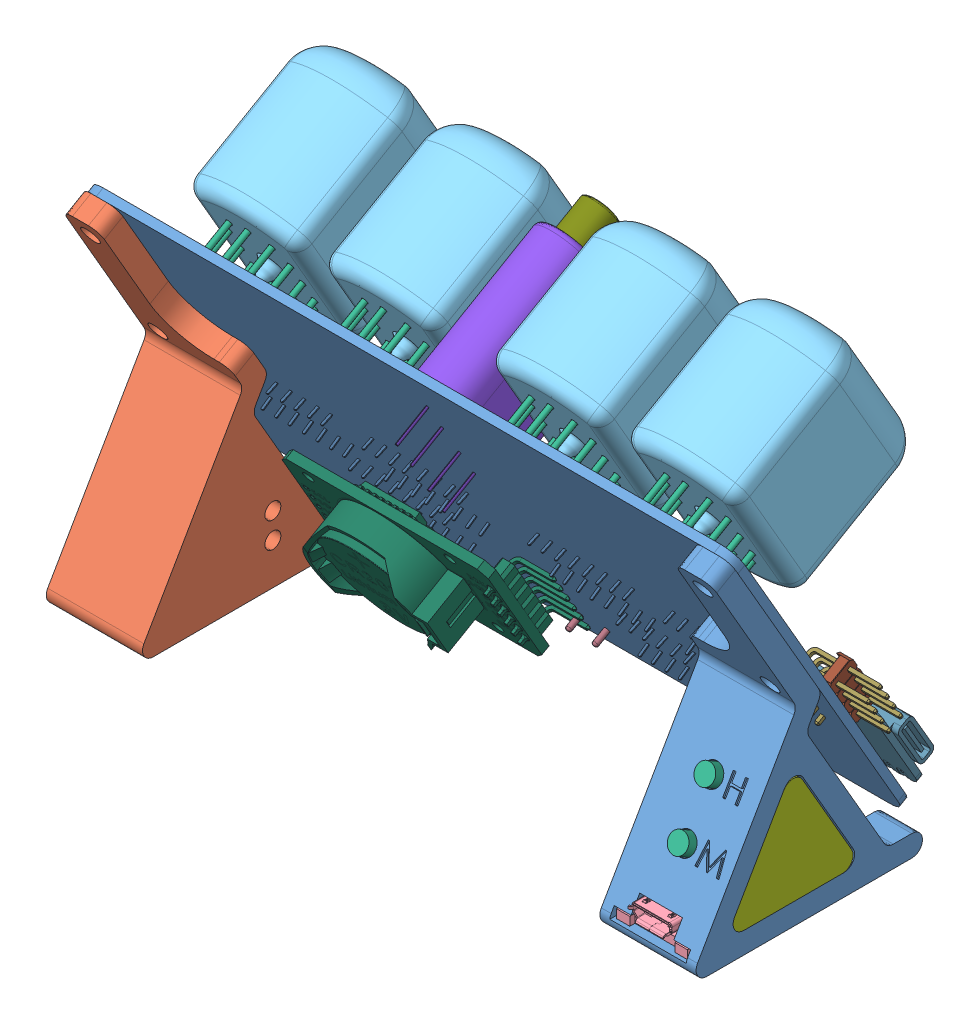
SolidWorks assembly assembly, configuration Défaut. Lengths in mm.
Overall size (130.66 87.93 77.4).
301 component instances, 62 part files, 34 mates.
Components (placement in the parent):
- board-1: board [Défaut] at (0 36.4164 17.774) x (-1 0 0) z (0 -0.866025 -0.5) size (127.16 50.53 67.27)
  - pcb-1: pcb [Défaut] at origin size (121.6 1.5 65.9)
  - IN-12A.stp-1: IN-12A.stp [Défaut] at (-40.9487 32.5 -15.5981) x (0 1 0) z (1 0 0) size (35 31 21)
    - 2.stp-1: 2.stp [Défaut] at origin size (2.7 24.17 15.83)
    - 3.stp-1: 3.stp [Défaut] at (-12.2 0 0) x (0 0 -1) z (-1 0 0) size (2 1.5 18.5)
    - 4.stp-1: 4.stp [Défaut] at (-12.2 0 0) x (0 0 1) z (-1 0 0) size (2 1.5 18.5)
    - 5.stp-1: 5.stp [Défaut] at (-12 0 0) x (0 0 -1) z (1 0 0) size (2.1 2.1 1)
    - 5.stp-2: 5.stp [Défaut] at (-10.8 0 0) x (0 0 -1) z (1 0 0) size (2.1 2.1 1)
    - 5.stp-3: 5.stp [Défaut] at (-9.6 0 0) x (0 0 -1) z (1 0 0) size (2.1 2.1 1)
    - 5.stp-4: 5.stp [Défaut] at (-8.4 0 0) x (0 0 -1) z (1 0 0) size (2.1 2.1 1)
    - 5.stp-5: 5.stp [Défaut] at (-7.2 0 0) x (0 0 -1) z (1 0 0) size (2.1 2.1 1)
    - 5.stp-6: 5.stp [Défaut] at (-6 0 0) x (0 0 -1) z (1 0 0) size (2.1 2.1 1)
    - 5.stp-7: 5.stp [Défaut] at (-4.8 0 0) x (0 0 -1) z (1 0 0) size (2.1 2.1 1)
    - 5.stp-8: 5.stp [Défaut] at (-3.6 0 0) x (0 0 -1) z (1 0 0) size (2.1 2.1 1)
    - 5.stp-9: 5.stp [Défaut] at (-2.4 0 0) x (0 0 -1) z (1 0 0) size (2.1 2.1 1)
    - 5.stp-10: 5.stp [Défaut] at (-1.2 0 0) x (0 0 -1) z (1 0 0) size (2.1 2.1 1)
    - 6.stp-1: 6.stp [Défaut] at (-11 16.1596 7.8778) x (0 -0.787778 0.61596) z (-1 0 0) size (2.1 2.1 1)
    - 7.stp-1: 7.stp [Défaut] at (-9.8 16.1596 7.8778) x (0 -0.787778 0.61596) z (-1 0 0) size (2.1 2.1 1)
    - 8.stp-1: 8.stp [Défaut] at (-8.6 16.1596 7.8778) x (0 -0.787778 0.61596) z (-1 0 0) size (2.1 2.1 1)
    - 9.stp-1: 9.stp [Défaut] at (-7.4 16.1596 7.8778) x (0 -0.787778 0.61596) z (-1 0 0) size (2.1 2.1 1)
    - 10.stp-1: 10.stp [Défaut] at (-6.2 16.1596 7.8778) x (0 -0.787778 0.61596) z (-1 0 0) size (2.1 2.1 1)
    - 11.stp-1: 11.stp [Défaut] at (-5 16.1596 7.8778) x (0 -0.787778 0.61596) z (-1 0 0) size (2.1 2.1 1)
    - 12.stp-1: 12.stp [Défaut] at (-3.8 16.1596 7.8778) x (0 -0.787778 0.61596) z (-1 0 0) size (2.1 2.1 1)
    - 13.stp-1: 13.stp [Défaut] at (-2.6 16.1596 7.8778) x (0 -0.787778 0.61596) z (-1 0 0) size (2.1 2.1 1)
    - 14.stp-1: 14.stp [Défaut] at (-1.4 16.1596 7.8778) x (0 -0.787778 0.61596) z (-1 0 0) size (2.1 2.1 1)
    - 15.stp-1: 15.stp [Défaut] at (-0.2 16.1596 7.8778) x (0 -0.787778 0.61596) z (-1 0 0) size (2.1 2.1 1)
    - 5.stp-11: 5.stp [Défaut] x (0 0 -1) z (1 0 0) size (2.1 2.1 1)
    - 5.stp-12: 5.stp [Défaut] at (-13.2 0 0) x (0 0 -1) z (1 0 0) size (2.1 2.1 1)
    - 16.stp-1: 16.stp [Défaut] at (1 16.1596 7.8778) x (0 -0.787778 0.61596) z (-1 0 0) size (2.1 2.1 1)
    - 17.stp-1: 17.stp [Défaut] at (-12.2 16.1596 7.8778) x (0 -0.787778 0.61596) z (-1 0 0) size (2.1 2.1 1)
    - 18.stp-1: 18.stp [Défaut] at (-13.2 0 0) x (0 0 -1) z (-1 0 0) size (15.83 24.17 12.28)
    - 19.stp-1: 19.stp [Défaut] x (1 0 0) z (0 1 0) size (1.51 1.46 20.68)
    - 20.stp-1: 20.stp [Défaut] at (1 0 0) size (4 22.27 2.42)
    - 21.stp-1: 21.stp [Défaut] at (-13.4 0 0) x (0 0 -1) z (-1 0 0) size (15.83 24.17 1)
    - 22.stp-1: 22.stp [Défaut] at (-14.4 0 0) x (0 0 -1) z (-1 0 0) size (15.83 27.29 2)
    - 23.stp-1: 23.stp [Défaut] x (0 0 -1) z (-1 0 0) size (21 31 33)
    - 24.stp-1: 24.stp [Défaut] x (0 0 -1) z (-1 0 0) size (1 1 15.5)
    - 24.stp-2: 24.stp [Défaut] at (0 -4.5 0) x (0 0 -1) z (-1 0 0) size (1 1 15.5)
    - 24.stp-3: 24.stp [Défaut] at (0 -8 -1.75) x (0 0 -1) z (-1 0 0) size (1 1 15.5)
    - 24.stp-4: 24.stp [Défaut] at (0 -9 -5.75) x (0 0 -1) z (-1 0 0) size (1 1 15.5)
    - 24.stp-5: 24.stp [Défaut] at (0 -8 -9.75) x (0 0 -1) z (-1 0 0) size (1 1 15.5)
    - 24.stp-6: 24.stp [Défaut] at (0 -4.5 -11.5) x (0 0 -1) z (-1 0 0) size (1 1 15.5)
    - 24.stp-7: 24.stp [Défaut] at (0 0 -11.5) x (0 0 -1) z (-1 0 0) size (1 1 15.5)
    - 24.stp-8: 24.stp [Défaut] at (0 4.5 -11.5) x (0 0 -1) z (-1 0 0) size (1 1 15.5)
    - 24.stp-9: 24.stp [Défaut] at (0 8 -9.75) x (0 0 -1) z (-1 0 0) size (1 1 15.5)
    - 24.stp-10: 24.stp [Défaut] at (0 9 -5.75) x (0 0 -1) z (-1 0 0) size (1 1 15.5)
    - 24.stp-11: 24.stp [Défaut] at (0 8 -1.75) x (0 0 -1) z (-1 0 0) size (1 1 15.5)
    - 24.stp-12: 24.stp [Défaut] at (0 4.5 0) x (0 0 -1) z (-1 0 0) size (1 1 15.5)
    - 25.stp-1: 25.stp [Défaut] at (-1.4 0 0) x (0 0 1) z (1 0 0) size (10.55 22 0.2)
    - 26.stp-1: 26.stp [Défaut] at (-2.6 0 0) x (0 0 1) z (1 0 0) size (11 22 0.2)
    - 27.stp-1: 27.stp [Défaut] at (-3.8 0 0) x (0 0 1) z (1 0 0) size (11 22 0.2)
    - 28.stp-1: 28.stp [Défaut] at (-5 0 0) x (0 0 1) z (1 0 0) size (10 22 0.2)
    - 29.stp-1: 29.stp [Défaut] at (-7.4 0 0) x (0 0 1) z (1 0 0) size (10 22 0.2)
    - 30.stp-1: 30.stp [Défaut] at (-9.6 0 0) x (0 0 -1) z (-1 0 0) size (10 22 0.2)
    - 31.stp-1: 31.stp [Défaut] at (-11 0 0) x (0 0 1) z (1 0 0) size (11 22 0.2)
    - 32.stp-1: 32.stp [Défaut] at (-12.2 0 0) x (0 0 1) z (1 0 0) size (2 22 0.2)
    - 33.stp-1: 33.stp [Défaut] at (-6 0 0) x (0 0 -1) z (-1 0 0) size (11 22 0.2)
    - 34.stp-1: 34.stp [Défaut] at (-8.6 0 0) x (0 0 1) z (1 0 0) size (10 22 0.2)
    - 1.stp-1: 1.stp [Défaut] at origin size (7.54 3.19 3.19)
    - 1-0.stp-1: 1-0.stp [Défaut] at origin size (11.99 9.11 6.32)
    - 1-1.stp-1: 1-1.stp [Défaut] at origin size (5.03 4.26 4.61)
    - 1-2.stp-1: 1-2.stp [Défaut] at origin size (8.17 8.42 6.65)
    - 1-3.stp-1: 1-3.stp [Défaut] at origin size (17.22 12.89 7.69)
    - 1-4.stp-1: 1-4.stp [Défaut] at origin size (13.11 12.81 7.39)
    - 1-5.stp-1: 1-5.stp [Défaut] at origin size (15.91 7.54 6.9)
    - 1-6.stp-1: 1-6.stp [Défaut] at origin size (10.39 4.47 4.23)
    - 1-7.stp-1: 1-7.stp [Défaut] at origin size (7.32 4.98 2.44)
    - 1-8.stp-1: 1-8.stp [Défaut] at origin size (10.29 4.36 5.63)
    - 1-9.stp-1: 1-9.stp [Défaut] at origin size (12.89 8.1 7.83)
  - IN-12A.stp-2: IN-12A.stp [Défaut] at (15.5408 32.5 -15.6508) x (0 1 0) z (1 0 0) size (35 31 21)
    - 2.stp-1: 2.stp [Défaut] at origin size (2.7 24.17 15.83)
    - 3.stp-1: 3.stp [Défaut] at (-12.2 0 0) x (0 0 -1) z (-1 0 0) size (2 1.5 18.5)
    - 4.stp-1: 4.stp [Défaut] at (-12.2 0 0) x (0 0 1) z (-1 0 0) size (2 1.5 18.5)
    - 5.stp-1: 5.stp [Défaut] at (-12 0 0) x (0 0 -1) z (1 0 0) size (2.1 2.1 1)
    - 5.stp-2: 5.stp [Défaut] at (-10.8 0 0) x (0 0 -1) z (1 0 0) size (2.1 2.1 1)
    - 5.stp-3: 5.stp [Défaut] at (-9.6 0 0) x (0 0 -1) z (1 0 0) size (2.1 2.1 1)
    - 5.stp-4: 5.stp [Défaut] at (-8.4 0 0) x (0 0 -1) z (1 0 0) size (2.1 2.1 1)
    - 5.stp-5: 5.stp [Défaut] at (-7.2 0 0) x (0 0 -1) z (1 0 0) size (2.1 2.1 1)
    - 5.stp-6: 5.stp [Défaut] at (-6 0 0) x (0 0 -1) z (1 0 0) size (2.1 2.1 1)
    - 5.stp-7: 5.stp [Défaut] at (-4.8 0 0) x (0 0 -1) z (1 0 0) size (2.1 2.1 1)
    - 5.stp-8: 5.stp [Défaut] at (-3.6 0 0) x (0 0 -1) z (1 0 0) size (2.1 2.1 1)
    - 5.stp-9: 5.stp [Défaut] at (-2.4 0 0) x (0 0 -1) z (1 0 0) size (2.1 2.1 1)
    - 5.stp-10: 5.stp [Défaut] at (-1.2 0 0) x (0 0 -1) z (1 0 0) size (2.1 2.1 1)
    - 6.stp-1: 6.stp [Défaut] at (-11 16.1596 7.8778) x (0 -0.787778 0.61596) z (-1 0 0) size (2.1 2.1 1)
    - 7.stp-1: 7.stp [Défaut] at (-9.8 16.1596 7.8778) x (0 -0.787778 0.61596) z (-1 0 0) size (2.1 2.1 1)
    - 8.stp-1: 8.stp [Défaut] at (-8.6 16.1596 7.8778) x (0 -0.787778 0.61596) z (-1 0 0) size (2.1 2.1 1)
    - 9.stp-1: 9.stp [Défaut] at (-7.4 16.1596 7.8778) x (0 -0.787778 0.61596) z (-1 0 0) size (2.1 2.1 1)
    - 10.stp-1: 10.stp [Défaut] at (-6.2 16.1596 7.8778) x (0 -0.787778 0.61596) z (-1 0 0) size (2.1 2.1 1)
    - 11.stp-1: 11.stp [Défaut] at (-5 16.1596 7.8778) x (0 -0.787778 0.61596) z (-1 0 0) size (2.1 2.1 1)
    - 12.stp-1: 12.stp [Défaut] at (-3.8 16.1596 7.8778) x (0 -0.787778 0.61596) z (-1 0 0) size (2.1 2.1 1)
    - 13.stp-1: 13.stp [Défaut] at (-2.6 16.1596 7.8778) x (0 -0.787778 0.61596) z (-1 0 0) size (2.1 2.1 1)
    - 14.stp-1: 14.stp [Défaut] at (-1.4 16.1596 7.8778) x (0 -0.787778 0.61596) z (-1 0 0) size (2.1 2.1 1)
    - 15.stp-1: 15.stp [Défaut] at (-0.2 16.1596 7.8778) x (0 -0.787778 0.61596) z (-1 0 0) size (2.1 2.1 1)
    - 5.stp-11: 5.stp [Défaut] x (0 0 -1) z (1 0 0) size (2.1 2.1 1)
    - 5.stp-12: 5.stp [Défaut] at (-13.2 0 0) x (0 0 -1) z (1 0 0) size (2.1 2.1 1)
    - 16.stp-1: 16.stp [Défaut] at (1 16.1596 7.8778) x (0 -0.787778 0.61596) z (-1 0 0) size (2.1 2.1 1)
    - 17.stp-1: 17.stp [Défaut] at (-12.2 16.1596 7.8778) x (0 -0.787778 0.61596) z (-1 0 0) size (2.1 2.1 1)
    - 18.stp-1: 18.stp [Défaut] at (-13.2 0 0) x (0 0 -1) z (-1 0 0) size (15.83 24.17 12.28)
    - 19.stp-1: 19.stp [Défaut] x (1 0 0) z (0 1 0) size (1.51 1.46 20.68)
    - 20.stp-1: 20.stp [Défaut] at (1 0 0) size (4 22.27 2.42)
    - 21.stp-1: 21.stp [Défaut] at (-13.4 0 0) x (0 0 -1) z (-1 0 0) size (15.83 24.17 1)
    - 22.stp-1: 22.stp [Défaut] at (-14.4 0 0) x (0 0 -1) z (-1 0 0) size (15.83 27.29 2)
    - 23.stp-1: 23.stp [Défaut] x (0 0 -1) z (-1 0 0) size (21 31 33)
    - 24.stp-1: 24.stp [Défaut] x (0 0 -1) z (-1 0 0) size (1 1 15.5)
    - 24.stp-2: 24.stp [Défaut] at (0 -4.5 0) x (0 0 -1) z (-1 0 0) size (1 1 15.5)
    - 24.stp-3: 24.stp [Défaut] at (0 -8 -1.75) x (0 0 -1) z (-1 0 0) size (1 1 15.5)
    - 24.stp-4: 24.stp [Défaut] at (0 -9 -5.75) x (0 0 -1) z (-1 0 0) size (1 1 15.5)
    - 24.stp-5: 24.stp [Défaut] at (0 -8 -9.75) x (0 0 -1) z (-1 0 0) size (1 1 15.5)
    - 24.stp-6: 24.stp [Défaut] at (0 -4.5 -11.5) x (0 0 -1) z (-1 0 0) size (1 1 15.5)
    - 24.stp-7: 24.stp [Défaut] at (0 0 -11.5) x (0 0 -1) z (-1 0 0) size (1 1 15.5)
    - 24.stp-8: 24.stp [Défaut] at (0 4.5 -11.5) x (0 0 -1) z (-1 0 0) size (1 1 15.5)
    - 24.stp-9: 24.stp [Défaut] at (0 8 -9.75) x (0 0 -1) z (-1 0 0) size (1 1 15.5)
    - 24.stp-10: 24.stp [Défaut] at (0 9 -5.75) x (0 0 -1) z (-1 0 0) size (1 1 15.5)
    - 24.stp-11: 24.stp [Défaut] at (0 8 -1.75) x (0 0 -1) z (-1 0 0) size (1 1 15.5)
    - 24.stp-12: 24.stp [Défaut] at (0 4.5 0) x (0 0 -1) z (-1 0 0) size (1 1 15.5)
    - 25.stp-1: 25.stp [Défaut] at (-1.4 0 0) x (0 0 1) z (1 0 0) size (10.55 22 0.2)
    - 26.stp-1: 26.stp [Défaut] at (-2.6 0 0) x (0 0 1) z (1 0 0) size (11 22 0.2)
    - 27.stp-1: 27.stp [Défaut] at (-3.8 0 0) x (0 0 1) z (1 0 0) size (11 22 0.2)
    - 28.stp-1: 28.stp [Défaut] at (-5 0 0) x (0 0 1) z (1 0 0) size (10 22 0.2)
    - 29.stp-1: 29.stp [Défaut] at (-7.4 0 0) x (0 0 1) z (1 0 0) size (10 22 0.2)
    - 30.stp-1: 30.stp [Défaut] at (-9.6 0 0) x (0 0 -1) z (-1 0 0) size (10 22 0.2)
    - 31.stp-1: 31.stp [Défaut] at (-11 0 0) x (0 0 1) z (1 0 0) size (11 22 0.2)
    - 32.stp-1: 32.stp [Défaut] at (-12.2 0 0) x (0 0 1) z (1 0 0) size (2 22 0.2)
    - 33.stp-1: 33.stp [Défaut] at (-6 0 0) x (0 0 -1) z (-1 0 0) size (11 22 0.2)
    - 34.stp-1: 34.stp [Défaut] at (-8.6 0 0) x (0 0 1) z (1 0 0) size (10 22 0.2)
    - 1.stp-1: 1.stp [Défaut] at origin size (7.54 3.19 3.19)
    - 1-0.stp-1: 1-0.stp [Défaut] at origin size (11.99 9.11 6.32)
    - 1-1.stp-1: 1-1.stp [Défaut] at origin size (5.03 4.26 4.61)
    - 1-2.stp-1: 1-2.stp [Défaut] at origin size (8.17 8.42 6.65)
    - 1-3.stp-1: 1-3.stp [Défaut] at origin size (17.22 12.89 7.69)
    - 1-4.stp-1: 1-4.stp [Défaut] at origin size (13.11 12.81 7.39)
    - 1-5.stp-1: 1-5.stp [Défaut] at origin size (15.91 7.54 6.9)
    - 1-6.stp-1: 1-6.stp [Défaut] at origin size (10.39 4.47 4.23)
    - 1-7.stp-1: 1-7.stp [Défaut] at origin size (7.32 4.98 2.44)
    - 1-8.stp-1: 1-8.stp [Défaut] at origin size (10.29 4.36 5.63)
    - 1-9.stp-1: 1-9.stp [Défaut] at origin size (12.89 8.1 7.83)
  - IN-12A.stp-3: IN-12A.stp [Défaut] at (-15.577 32.5 -15.4564) x (0 1 0) z (1 0 0) size (35 31 21)
    - 2.stp-1: 2.stp [Défaut] at origin size (2.7 24.17 15.83)
    - 3.stp-1: 3.stp [Défaut] at (-12.2 0 0) x (0 0 -1) z (-1 0 0) size (2 1.5 18.5)
    - 4.stp-1: 4.stp [Défaut] at (-12.2 0 0) x (0 0 1) z (-1 0 0) size (2 1.5 18.5)
    - 5.stp-1: 5.stp [Défaut] at (-12 0 0) x (0 0 -1) z (1 0 0) size (2.1 2.1 1)
    - 5.stp-2: 5.stp [Défaut] at (-10.8 0 0) x (0 0 -1) z (1 0 0) size (2.1 2.1 1)
    - 5.stp-3: 5.stp [Défaut] at (-9.6 0 0) x (0 0 -1) z (1 0 0) size (2.1 2.1 1)
    - 5.stp-4: 5.stp [Défaut] at (-8.4 0 0) x (0 0 -1) z (1 0 0) size (2.1 2.1 1)
    - 5.stp-5: 5.stp [Défaut] at (-7.2 0 0) x (0 0 -1) z (1 0 0) size (2.1 2.1 1)
    - 5.stp-6: 5.stp [Défaut] at (-6 0 0) x (0 0 -1) z (1 0 0) size (2.1 2.1 1)
    - 5.stp-7: 5.stp [Défaut] at (-4.8 0 0) x (0 0 -1) z (1 0 0) size (2.1 2.1 1)
    - 5.stp-8: 5.stp [Défaut] at (-3.6 0 0) x (0 0 -1) z (1 0 0) size (2.1 2.1 1)
    - 5.stp-9: 5.stp [Défaut] at (-2.4 0 0) x (0 0 -1) z (1 0 0) size (2.1 2.1 1)
    - 5.stp-10: 5.stp [Défaut] at (-1.2 0 0) x (0 0 -1) z (1 0 0) size (2.1 2.1 1)
    - 6.stp-1: 6.stp [Défaut] at (-11 16.1596 7.8778) x (0 -0.787778 0.61596) z (-1 0 0) size (2.1 2.1 1)
    - 7.stp-1: 7.stp [Défaut] at (-9.8 16.1596 7.8778) x (0 -0.787778 0.61596) z (-1 0 0) size (2.1 2.1 1)
    - 8.stp-1: 8.stp [Défaut] at (-8.6 16.1596 7.8778) x (0 -0.787778 0.61596) z (-1 0 0) size (2.1 2.1 1)
    - 9.stp-1: 9.stp [Défaut] at (-7.4 16.1596 7.8778) x (0 -0.787778 0.61596) z (-1 0 0) size (2.1 2.1 1)
    - 10.stp-1: 10.stp [Défaut] at (-6.2 16.1596 7.8778) x (0 -0.787778 0.61596) z (-1 0 0) size (2.1 2.1 1)
    - 11.stp-1: 11.stp [Défaut] at (-5 16.1596 7.8778) x (0 -0.787778 0.61596) z (-1 0 0) size (2.1 2.1 1)
    - 12.stp-1: 12.stp [Défaut] at (-3.8 16.1596 7.8778) x (0 -0.787778 0.61596) z (-1 0 0) size (2.1 2.1 1)
    - 13.stp-1: 13.stp [Défaut] at (-2.6 16.1596 7.8778) x (0 -0.787778 0.61596) z (-1 0 0) size (2.1 2.1 1)
    - 14.stp-1: 14.stp [Défaut] at (-1.4 16.1596 7.8778) x (0 -0.787778 0.61596) z (-1 0 0) size (2.1 2.1 1)
    - 15.stp-1: 15.stp [Défaut] at (-0.2 16.1596 7.8778) x (0 -0.787778 0.61596) z (-1 0 0) size (2.1 2.1 1)
    - 5.stp-11: 5.stp [Défaut] x (0 0 -1) z (1 0 0) size (2.1 2.1 1)
    - 5.stp-12: 5.stp [Défaut] at (-13.2 0 0) x (0 0 -1) z (1 0 0) size (2.1 2.1 1)
    - 16.stp-1: 16.stp [Défaut] at (1 16.1596 7.8778) x (0 -0.787778 0.61596) z (-1 0 0) size (2.1 2.1 1)
    - 17.stp-1: 17.stp [Défaut] at (-12.2 16.1596 7.8778) x (0 -0.787778 0.61596) z (-1 0 0) size (2.1 2.1 1)
    - 18.stp-1: 18.stp [Défaut] at (-13.2 0 0) x (0 0 -1) z (-1 0 0) size (15.83 24.17 12.28)
    - 19.stp-1: 19.stp [Défaut] x (1 0 0) z (0 1 0) size (1.51 1.46 20.68)
    - 20.stp-1: 20.stp [Défaut] at (1 0 0) size (4 22.27 2.42)
    - 21.stp-1: 21.stp [Défaut] at (-13.4 0 0) x (0 0 -1) z (-1 0 0) size (15.83 24.17 1)
    - 22.stp-1: 22.stp [Défaut] at (-14.4 0 0) x (0 0 -1) z (-1 0 0) size (15.83 27.29 2)
    - 23.stp-1: 23.stp [Défaut] x (0 0 -1) z (-1 0 0) size (21 31 33)
    - 24.stp-1: 24.stp [Défaut] x (0 0 -1) z (-1 0 0) size (1 1 15.5)
    - 24.stp-2: 24.stp [Défaut] at (0 -4.5 0) x (0 0 -1) z (-1 0 0) size (1 1 15.5)
    - 24.stp-3: 24.stp [Défaut] at (0 -8 -1.75) x (0 0 -1) z (-1 0 0) size (1 1 15.5)
    - 24.stp-4: 24.stp [Défaut] at (0 -9 -5.75) x (0 0 -1) z (-1 0 0) size (1 1 15.5)
    - 24.stp-5: 24.stp [Défaut] at (0 -8 -9.75) x (0 0 -1) z (-1 0 0) size (1 1 15.5)
    - 24.stp-6: 24.stp [Défaut] at (0 -4.5 -11.5) x (0 0 -1) z (-1 0 0) size (1 1 15.5)
    - 24.stp-7: 24.stp [Défaut] at (0 0 -11.5) x (0 0 -1) z (-1 0 0) size (1 1 15.5)
    - 24.stp-8: 24.stp [Défaut] at (0 4.5 -11.5) x (0 0 -1) z (-1 0 0) size (1 1 15.5)
    - 24.stp-9: 24.stp [Défaut] at (0 8 -9.75) x (0 0 -1) z (-1 0 0) size (1 1 15.5)
    - 24.stp-10: 24.stp [Défaut] at (0 9 -5.75) x (0 0 -1) z (-1 0 0) size (1 1 15.5)
    - 24.stp-11: 24.stp [Défaut] at (0 8 -1.75) x (0 0 -1) z (-1 0 0) size (1 1 15.5)
    - 24.stp-12: 24.stp [Défaut] at (0 4.5 0) x (0 0 -1) z (-1 0 0) size (1 1 15.5)
    - 25.stp-1: 25.stp [Défaut] at (-1.4 0 0) x (0 0 1) z (1 0 0) size (10.55 22 0.2)
    - 26.stp-1: 26.stp [Défaut] at (-2.6 0 0) x (0 0 1) z (1 0 0) size (11 22 0.2)
    - 27.stp-1: 27.stp [Défaut] at (-3.8 0 0) x (0 0 1) z (1 0 0) size (11 22 0.2)
    - 28.stp-1: 28.stp [Défaut] at (-5 0 0) x (0 0 1) z (1 0 0) size (10 22 0.2)
    - 29.stp-1: 29.stp [Défaut] at (-7.4 0 0) x (0 0 1) z (1 0 0) size (10 22 0.2)
    - 30.stp-1: 30.stp [Défaut] at (-9.6 0 0) x (0 0 -1) z (-1 0 0) size (10 22 0.2)
    - 31.stp-1: 31.stp [Défaut] at (-11 0 0) x (0 0 1) z (1 0 0) size (11 22 0.2)
    - 32.stp-1: 32.stp [Défaut] at (-12.2 0 0) x (0 0 1) z (1 0 0) size (2 22 0.2)
    - 33.stp-1: 33.stp [Défaut] at (-6 0 0) x (0 0 -1) z (-1 0 0) size (11 22 0.2)
    - 34.stp-1: 34.stp [Défaut] at (-8.6 0 0) x (0 0 1) z (1 0 0) size (10 22 0.2)
    - 1.stp-1: 1.stp [Défaut] at origin size (7.54 3.19 3.19)
    - 1-0.stp-1: 1-0.stp [Défaut] at origin size (11.99 9.11 6.32)
    - 1-1.stp-1: 1-1.stp [Défaut] at origin size (5.03 4.26 4.61)
    - 1-2.stp-1: 1-2.stp [Défaut] at origin size (8.17 8.42 6.65)
    - 1-3.stp-1: 1-3.stp [Défaut] at origin size (17.22 12.89 7.69)
    - 1-4.stp-1: 1-4.stp [Défaut] at origin size (13.11 12.81 7.39)
    - 1-5.stp-1: 1-5.stp [Défaut] at origin size (15.91 7.54 6.9)
    - 1-6.stp-1: 1-6.stp [Défaut] at origin size (10.39 4.47 4.23)
    - 1-7.stp-1: 1-7.stp [Défaut] at origin size (7.32 4.98 2.44)
    - 1-8.stp-1: 1-8.stp [Défaut] at origin size (10.29 4.36 5.63)
    - 1-9.stp-1: 1-9.stp [Défaut] at origin size (12.89 8.1 7.83)
  - IN-12A.stp-4: IN-12A.stp [Défaut] at (40.934 32.5 -15.666) x (0 1 0) z (1 0 0) size (35 31 21)
    - 2.stp-1: 2.stp [Défaut] at origin size (2.7 24.17 15.83)
    - 3.stp-1: 3.stp [Défaut] at (-12.2 0 0) x (0 0 -1) z (-1 0 0) size (2 1.5 18.5)
    - 4.stp-1: 4.stp [Défaut] at (-12.2 0 0) x (0 0 1) z (-1 0 0) size (2 1.5 18.5)
    - 5.stp-1: 5.stp [Défaut] at (-12 0 0) x (0 0 -1) z (1 0 0) size (2.1 2.1 1)
    - 5.stp-2: 5.stp [Défaut] at (-10.8 0 0) x (0 0 -1) z (1 0 0) size (2.1 2.1 1)
    - 5.stp-3: 5.stp [Défaut] at (-9.6 0 0) x (0 0 -1) z (1 0 0) size (2.1 2.1 1)
    - 5.stp-4: 5.stp [Défaut] at (-8.4 0 0) x (0 0 -1) z (1 0 0) size (2.1 2.1 1)
    - 5.stp-5: 5.stp [Défaut] at (-7.2 0 0) x (0 0 -1) z (1 0 0) size (2.1 2.1 1)
    - 5.stp-6: 5.stp [Défaut] at (-6 0 0) x (0 0 -1) z (1 0 0) size (2.1 2.1 1)
    - 5.stp-7: 5.stp [Défaut] at (-4.8 0 0) x (0 0 -1) z (1 0 0) size (2.1 2.1 1)
    - 5.stp-8: 5.stp [Défaut] at (-3.6 0 0) x (0 0 -1) z (1 0 0) size (2.1 2.1 1)
    - 5.stp-9: 5.stp [Défaut] at (-2.4 0 0) x (0 0 -1) z (1 0 0) size (2.1 2.1 1)
    - 5.stp-10: 5.stp [Défaut] at (-1.2 0 0) x (0 0 -1) z (1 0 0) size (2.1 2.1 1)
    - 6.stp-1: 6.stp [Défaut] at (-11 16.1596 7.8778) x (0 -0.787778 0.61596) z (-1 0 0) size (2.1 2.1 1)
    - 7.stp-1: 7.stp [Défaut] at (-9.8 16.1596 7.8778) x (0 -0.787778 0.61596) z (-1 0 0) size (2.1 2.1 1)
    - 8.stp-1: 8.stp [Défaut] at (-8.6 16.1596 7.8778) x (0 -0.787778 0.61596) z (-1 0 0) size (2.1 2.1 1)
    - 9.stp-1: 9.stp [Défaut] at (-7.4 16.1596 7.8778) x (0 -0.787778 0.61596) z (-1 0 0) size (2.1 2.1 1)
    - 10.stp-1: 10.stp [Défaut] at (-6.2 16.1596 7.8778) x (0 -0.787778 0.61596) z (-1 0 0) size (2.1 2.1 1)
    - 11.stp-1: 11.stp [Défaut] at (-5 16.1596 7.8778) x (0 -0.787778 0.61596) z (-1 0 0) size (2.1 2.1 1)
    - 12.stp-1: 12.stp [Défaut] at (-3.8 16.1596 7.8778) x (0 -0.787778 0.61596) z (-1 0 0) size (2.1 2.1 1)
    - 13.stp-1: 13.stp [Défaut] at (-2.6 16.1596 7.8778) x (0 -0.787778 0.61596) z (-1 0 0) size (2.1 2.1 1)
    - 14.stp-1: 14.stp [Défaut] at (-1.4 16.1596 7.8778) x (0 -0.787778 0.61596) z (-1 0 0) size (2.1 2.1 1)
    - 15.stp-1: 15.stp [Défaut] at (-0.2 16.1596 7.8778) x (0 -0.787778 0.61596) z (-1 0 0) size (2.1 2.1 1)
    - 5.stp-11: 5.stp [Défaut] x (0 0 -1) z (1 0 0) size (2.1 2.1 1)
    - 5.stp-12: 5.stp [Défaut] at (-13.2 0 0) x (0 0 -1) z (1 0 0) size (2.1 2.1 1)
    - 16.stp-1: 16.stp [Défaut] at (1 16.1596 7.8778) x (0 -0.787778 0.61596) z (-1 0 0) size (2.1 2.1 1)
    - 17.stp-1: 17.stp [Défaut] at (-12.2 16.1596 7.8778) x (0 -0.787778 0.61596) z (-1 0 0) size (2.1 2.1 1)
    - 18.stp-1: 18.stp [Défaut] at (-13.2 0 0) x (0 0 -1) z (-1 0 0) size (15.83 24.17 12.28)
    - 19.stp-1: 19.stp [Défaut] x (1 0 0) z (0 1 0) size (1.51 1.46 20.68)
    - 20.stp-1: 20.stp [Défaut] at (1 0 0) size (4 22.27 2.42)
    - 21.stp-1: 21.stp [Défaut] at (-13.4 0 0) x (0 0 -1) z (-1 0 0) size (15.83 24.17 1)
    - 22.stp-1: 22.stp [Défaut] at (-14.4 0 0) x (0 0 -1) z (-1 0 0) size (15.83 27.29 2)
    - 23.stp-1: 23.stp [Défaut] x (0 0 -1) z (-1 0 0) size (21 31 33)
    - 24.stp-1: 24.stp [Défaut] x (0 0 -1) z (-1 0 0) size (1 1 15.5)
    - 24.stp-2: 24.stp [Défaut] at (0 -4.5 0) x (0 0 -1) z (-1 0 0) size (1 1 15.5)
    - 24.stp-3: 24.stp [Défaut] at (0 -8 -1.75) x (0 0 -1) z (-1 0 0) size (1 1 15.5)
    - 24.stp-4: 24.stp [Défaut] at (0 -9 -5.75) x (0 0 -1) z (-1 0 0) size (1 1 15.5)
    - 24.stp-5: 24.stp [Défaut] at (0 -8 -9.75) x (0 0 -1) z (-1 0 0) size (1 1 15.5)
    - 24.stp-6: 24.stp [Défaut] at (0 -4.5 -11.5) x (0 0 -1) z (-1 0 0) size (1 1 15.5)
    - 24.stp-7: 24.stp [Défaut] at (0 0 -11.5) x (0 0 -1) z (-1 0 0) size (1 1 15.5)
    - 24.stp-8: 24.stp [Défaut] at (0 4.5 -11.5) x (0 0 -1) z (-1 0 0) size (1 1 15.5)
    - 24.stp-9: 24.stp [Défaut] at (0 8 -9.75) x (0 0 -1) z (-1 0 0) size (1 1 15.5)
    - 24.stp-10: 24.stp [Défaut] at (0 9 -5.75) x (0 0 -1) z (-1 0 0) size (1 1 15.5)
    - 24.stp-11: 24.stp [Défaut] at (0 8 -1.75) x (0 0 -1) z (-1 0 0) size (1 1 15.5)
    - 24.stp-12: 24.stp [Défaut] at (0 4.5 0) x (0 0 -1) z (-1 0 0) size (1 1 15.5)
    - 25.stp-1: 25.stp [Défaut] at (-1.4 0 0) x (0 0 1) z (1 0 0) size (10.55 22 0.2)
    - 26.stp-1: 26.stp [Défaut] at (-2.6 0 0) x (0 0 1) z (1 0 0) size (11 22 0.2)
    - 27.stp-1: 27.stp [Défaut] at (-3.8 0 0) x (0 0 1) z (1 0 0) size (11 22 0.2)
    - 28.stp-1: 28.stp [Défaut] at (-5 0 0) x (0 0 1) z (1 0 0) size (10 22 0.2)
    - 29.stp-1: 29.stp [Défaut] at (-7.4 0 0) x (0 0 1) z (1 0 0) size (10 22 0.2)
    - 30.stp-1: 30.stp [Défaut] at (-9.6 0 0) x (0 0 -1) z (-1 0 0) size (10 22 0.2)
    - 31.stp-1: 31.stp [Défaut] at (-11 0 0) x (0 0 1) z (1 0 0) size (11 22 0.2)
    - 32.stp-1: 32.stp [Défaut] at (-12.2 0 0) x (0 0 1) z (1 0 0) size (2 22 0.2)
    - 33.stp-1: 33.stp [Défaut] at (-6 0 0) x (0 0 -1) z (-1 0 0) size (11 22 0.2)
    - 34.stp-1: 34.stp [Défaut] at (-8.6 0 0) x (0 0 1) z (1 0 0) size (10 22 0.2)
    - 1.stp-1: 1.stp [Défaut] at origin size (7.54 3.19 3.19)
    - 1-0.stp-1: 1-0.stp [Défaut] at origin size (11.99 9.11 6.32)
    - 1-1.stp-1: 1-1.stp [Défaut] at origin size (5.03 4.26 4.61)
    - 1-2.stp-1: 1-2.stp [Défaut] at origin size (8.17 8.42 6.65)
    - 1-3.stp-1: 1-3.stp [Défaut] at origin size (17.22 12.89 7.69)
    - 1-4.stp-1: 1-4.stp [Défaut] at origin size (13.11 12.81 7.39)
    - 1-5.stp-1: 1-5.stp [Défaut] at origin size (15.91 7.54 6.9)
    - 1-6.stp-1: 1-6.stp [Défaut] at origin size (10.39 4.47 4.23)
    - 1-7.stp-1: 1-7.stp [Défaut] at origin size (7.32 4.98 2.44)
    - 1-8.stp-1: 1-8.stp [Défaut] at origin size (10.29 4.36 5.63)
    - 1-9.stp-1: 1-9.stp [Défaut] at origin size (12.89 8.1 7.83)
  - DIP18N.step-1: DIP18N.step [Défaut] at (-50.7835 3.7087 35.4382) x (0 0 1) z (-1 0 0) size (8.53 6.85 19.5)
  - DIP18N.step-2: DIP18N.step [Défaut] at (31.1067 3.7087 35.4997) x (0 0 1) z (-1 0 0) size (8.53 6.85 19.5)
  - DIP18N.step-3: DIP18N.step [Défaut] at (5.6608 3.7087 35.5611) x (0 0 1) z (-1 0 0) size (8.53 6.85 19.5)
  - DIP18N.step-4: DIP18N.step [Défaut] at (-25.3559 3.7087 35.5399) x (0 0 1) z (-1 0 0) size (8.53 6.85 19.5)
  - DS1022-2x4RF11.stp-1: DS1022-2x4RF11.stp [Défaut] at (-56.1796 1.5 3.5604) x (0 0 1) z (0 1 0) size (10.16 13.04 8)
    - eBom-prt0.stp-1: eBom-prt0.stp [Défaut] at origin size (10.16 2.5 5)
    - eBom-prt1.stp-1: eBom-prt1.stp [Défaut] at origin size (0.64 13.04 7.09)
    - eBom-prt1.stp-2: eBom-prt1.stp [Défaut] at (2.54 0 0) size (0.64 13.04 7.09)
    - eBom-prt1.stp-3: eBom-prt1.stp [Défaut] at (5.08 0 0) size (0.64 13.04 7.09)
    - eBom-prt1.stp-4: eBom-prt1.stp [Défaut] at (7.62 0 0) size (0.64 13.04 7.09)
  - DIP18N.step-5: DIP18N.step [Défaut] at (-15.751 3.7087 -7.8923) x (0.008727 0 -0.999962) z (0.999962 0 0.008727) size (8.53 6.85 19.5)
  - DIP18N.step-6: DIP18N.step [Défaut] at (34.3108 3.7087 -7.8662) x (0.008727 0 -0.999962) z (0.999962 0 0.008727) size (8.53 6.85 19.5)
  - Screw Terminal Block 5mm-2: Screw Terminal Block 5mm [Valor predeterminado] at (0.4217 1.5 23.933) x (-0.999962 0 -0.008727) z (0.008727 0 -0.999962) size (10.6 16.9 9)
  - Seeeduino Xiao.step-1: Seeeduino Xiao.step [Défaut] at (-88.5187 11.44 25.9289) x (-0.008727 0 0.999962) z (-0.999962 0 -0.008727) size (17.8 4.27 22.5)
  - DS3231 RTC.step-1: DS3231 RTC.step [Défaut] at (21.2627 -4.62 22.922) x (1 0 0) z (0 1 0) size (44.75 22.8 13.53)
  - INS1.STEP-1: INS1.STEP [Défaut] at (0 18.5 -21.8057) x (0 0 1) z (-1 0 0) size (7.01 43.17 6.51)
    - INS1-Glask_rper_01.STEP-1: INS1-Glask_rper_01.STEP [Défaut] at origin size (7.01 28.6 6.51)
    - INS1_Inlay_01.STEP-1: INS1_Inlay_01.STEP [Défaut] at (0 5.1 0) size (6 41.77 5.25)
  - INS1.STEP-2: INS1.STEP [Défaut] at (0 18.5 -9.8057) x (0 0 1) z (-1 0 0) size (7.01 43.17 6.51)
    - INS1-Glask_rper_01.STEP-1: INS1-Glask_rper_01.STEP [Défaut] at origin size (7.01 28.6 6.51)
    - INS1_Inlay_01.STEP-1: INS1_Inlay_01.STEP [Défaut] at (0 5.1 0) size (6 41.77 5.25)
- hv-cover-1: hv-cover [Défaut] at (-59.2 20.5901 2.2859) x (-1 0 0) z (0 0.5 -0.866025) size (20.6 23 8)
- leg-left-1: leg-left [Défaut] at (42.8 0 -3.251) size (18 64.95 42.38)
- leg-right-1: leg-right [Défaut] at (-60.8 0 -3.251) size (18 64.95 42.38)
- plate-right-1: plate-right [Défaut] at (-56.7 4.2252 22.2905) x (0 0 1) z (-1 0 0) size (21.97 19.56 3.5)
- Micro-USB_breakout.step-1: Micro-USB_breakout.step [Défaut] at (58.45 3.8 39.8564) x (0 0 -1) z (0 1 0) size (16.21 13.3 4.6)
- Push Button WHITE-1: Push Button WHITE [Default] at (-55.4 10.1 22.2905) x (0 0 1) z (0 -1 0) size (13 15.4 13)
- 6x6 mm-1: 6x6 mm [Défaut] at (51.8 13.5942 31.9004) x (1 0 0) z (0 -0.866025 0.5) size (8.15 10.4 6.02)
- 6x6 mm-2: 6x6 mm [Défaut] at (51.8 22.2545 26.9004) x (1 0 0) z (0 -0.866025 0.5) size (8.15 10.4 6.02)
- plate-left-1: plate-left [Défaut] at (60.8 14.9985 28.7802) x (0 0.866025 -0.5) z (-1 0 0) size (22.47 20 3.5)
- indic-holder-1: indic-holder [Défaut] at (0 50.8545 24.3779) x (1 0 0) z (0 0.866025 0.5) size (10.8 28.02 23.8)
Mates (geometry in assembly coordinates):
- Coïncidente11: coincident anti-aligned: plane of nixie-display-1 through (0 36.4164 17.774) normal (-1 0 0)
- Coïncidente14: coincident: line of nixie-display-1/pcb-1 through (115.6 57.8 8.6308) axis (0 -1 0)
- Coïncidente15: coincident anti-aligned: plane of nixie-display-1/pcb-1 through (0 36.4164 17.774) normal (0 -0.5 0.866025); plane of leg-io-1 through (60.8 64.9519 34.249) normal (0 0.5 -0.866025)
- Coïncidente17: coincident anti-aligned: plane of leg-io-1 through (60.8 0 42.0584) normal (0 -1 0)
- Coïncidente18: coincident anti-aligned: line of nixie-display-1/pcb-1 through (-57.8 64.9519 34.249) axis (1 0 0); line of leg-io-1 through (58.8 64.9519 34.249) axis (-1 0 0)
- Coïncidente19: coincident anti-aligned: plane of leg-io-1 through (42.8 2.2 -3.251) normal (0 1 0); plane of Micro-USB_breakout.step-1 through (51.8039 2.2 32.1496) normal (0 -1 0)
- Coïncidente20: coincident anti-aligned: plane of leg-io-1 through (44.65 2.2 24.249) normal (0 0 1); plane of Micro-USB_breakout.step-1 through (58.45 3.8 24.249) normal (0 0 -1)
- Largeur2: width anti-aligned: plane of leg-io-1 through (44.65 2.2 42.0584) normal (1 0 0); plane of leg-io-1 through (58.95 2.2 42.0584) normal (-1 0 0); plane of Micro-USB_breakout.step-1 through (45.15 3.8 24.249) normal (-1 0 0); plane of Micro-USB_breakout.step-1 through (58.45 3.8 39.8564) normal (1 0 0)
- Coaxiale1: concentric anti-aligned: cylinder of leg-io-1 through (51.8 3.6343 -5.3508) axis (0 0.5 0.866025) radius 2; cylinder of 6x6 mm-2 through (51.8 22.2545 26.9004) axis (0 -0.5 -0.866025) radius 1.82
- Coïncidente23: coincident anti-aligned: plane of leg-io-1 through (42.8 18.6195 28.999) normal (0 -0.5 -0.866025); plane of 6x6 mm-2 through (51.8 22.2545 26.9004) normal (0 0.5 0.866025)
- Parallèle2: parallel aligned: plane of leg-io-1 through (60.8 0 -3.251) normal (1 0 0); plane of 6x6 mm-2 through (54.8 24.8526 25.4004) normal (1 0 0)
- Coïncidente25: coincident anti-aligned: plane of leg-io-1 through (42.8 18.6195 28.999) normal (0 -0.5 -0.866025); plane of 6x6 mm-1 through (51.8 13.5942 31.9004) normal (0 0.5 0.866025)
- Coaxiale2: concentric anti-aligned: cylinder of leg-io-1 through (51.8 -5.026 -0.3508) axis (0 0.5 0.866025) radius 2; cylinder of 6x6 mm-1 through (51.8 13.5942 31.9004) axis (0 -0.5 -0.866025) radius 1.82
- Coïncidente26: coincident aligned: plane of 6x6 mm-1 through (54.8 16.1923 30.4004) normal (1 0 0); plane of 6x6 mm-2 through (54.8 24.8526 25.4004) normal (1 0 0)
- Coïncidente27: coincident anti-aligned: plane of nixie-display-1/pcb-1 through (0 36.4164 17.774) normal (0 -0.5 0.866025); plane of leg-button-1 through (-42.8 64.9519 34.249) normal (0 0.5 -0.866025)
- Coïncidente28: coincident aligned: plane of leg-io-1 through (60.8 0 42.0584) normal (0 -1 0); plane of leg-button-1 through (-42.8 0 42.0584) normal (0 -1 0)
- Coïncidente29: coincident aligned: plane of nixie-display-1/pcb-1 through (-60.8 65.7019 32.95) normal (-1 0 0); plane of leg-button-1 through (-60.8 0 -3.251) normal (-1 0 0)
- Coïncidente30: coincident aligned: plane of nixie-display-1/pcb-1 through (60.8 65.7019 32.95) normal (1 0 0); plane of leg-io-1 through (60.8 0 -3.251) normal (1 0 0)
- Parallèle3: parallel aligned: plane of Push Button WHITE-1 through (-64.3 4.9 22.2905) normal (-1 0 0); plane of leg-button-1 through (-60.8 0 -3.251) normal (-1 0 0)
- Largeur5: width aligned: plane of Push Button WHITE-1 through (-52.4 4.13 16.3205) normal (0 -1 0); plane of Push Button WHITE-1 through (-52.4 16.07 16.3205) normal (0 1 0); plane of leg-button-1 through (-52.4 16.2 17.1905) normal (0 -1 0); plane of leg-button-1 through (-52.4 4 17.1905) normal (0 1 0)
- Coïncidente35: coincident anti-aligned: plane of Push Button WHITE-1 through (-52.4 10.1 22.2905) normal (1 0 0); plane of leg-button-1 through (-52.4 12.5 28.3905) normal (-1 0 0)
- Largeur6: width anti-aligned: plane of Push Button WHITE-1 through (-52.4 16.07 16.3205) normal (0 0 -1); plane of Push Button WHITE-1 through (-52.4 16.07 28.2605) normal (0 0 1); plane of leg-button-1 through (-52.4 6.8 16.1905) normal (0 0 1); plane of leg-button-1 through (-52.4 6.8 28.3905) normal (0 0 -1)
- Largeur3: width anti-aligned: plane of button-plate-1 through (-65.8569 12.1 24.2905) normal (0 -1 0); plane of button-plate-1 through (-65.8569 8.1 24.2905) normal (0 1 0); plane of Push Button WHITE-1 through (-59.6 12.025 20.5655) normal (0 1 0); plane of Push Button WHITE-1 through (-59.6 8.175 20.5655) normal (0 -1 0)
- Largeur4: width anti-aligned: plane of button-plate-1 through (-65.8569 12.1 20.2905) normal (0 0 1); plane of button-plate-1 through (-65.8569 12.1 24.2905) normal (0 0 -1); plane of Push Button WHITE-1 through (-59.6 11.825 20.3655) normal (0 0 -1); plane of Push Button WHITE-1 through (-59.6 11.825 24.2155) normal (0 0 1)
- Coïncidente40: coincident anti-aligned: plane of Push Button WHITE-1 through (-59.6 11.825 20.5655) normal (-1 0 0); plane of button-plate-1 through (-59.6 4.2252 22.2905) normal (1 0 0)
- Coïncidente41: coincident anti-aligned: plane of nixie-display-1/pcb-1 through (0 37.1664 16.475) normal (0 0.5 -0.866025); plane of cover-1 through (-60.8 28.5494 11.5) normal (0 -0.5 0.866025)
- Coïncidente42: coincident aligned: plane of nixie-display-1/pcb-1 through (-60.8 65.7019 32.95) normal (-1 0 0); plane of cover-1 through (-60.8 20.5901 2.2859) normal (-1 0 0)
- Coïncidente43: coincident aligned: plane of nixie-display-1/pcb-1 through (60.8 8.6308 0) normal (0 -0.866025 -0.5); plane of cover-1 through (-60.8 12.6308 -6.9282) normal (0 -0.866025 -0.5)
- Coïncidente44: coincident aligned: plane of leg-left-1 through (60.8 0 -3.251) normal (1 0 0); plane of left-plate-1 through (60.8 14.9985 28.7802) normal (1 0 0)
- Coïncidente45: coincident anti-aligned: plane of leg-left-1 through (60.8 4 35.1302) normal (0 1 0); plane of left-plate-1 through (57.3 4 9.7302) normal (0 -1 0)
- Coïncidente46: coincident anti-aligned: plane of leg-left-1 through (60.8 26.2391 22.2905) normal (0 -0.5 -0.866025); plane of left-plate-1 through (57.3 4 35.1302) normal (0 0.5 0.866025)
- Coïncidente47: coincident: plane of board-1/pcb-1 through (0 37.1664 16.475) normal (0 0.5 -0.866025); plane of indic-holder-1 through (0 45.2254 21.1279) normal (0 -0.5 0.866025)
- Coaxiale3: concentric: cylinder of board-1/INS1.STEP-1/INS1-Glask_rper_01.STEP-1 through (0 73.5507 -2.933) axis (0 -0.5 0.866025) radius 3.25; cylinder of indic-holder-1 through (0 56.0507 27.3779) axis (0 0.5 -0.866025) radius 3.5
- Coaxiale4: concentric anti-aligned: cylinder of board-1/INS1.STEP-2/INS1-Glask_rper_01.STEP-1 through (0 63.1584 -8.933) axis (0 -0.5 0.866025) radius 3.25; cylinder of indic-holder-1 through (0 45.6584 21.3779) axis (0 0.5 -0.866025) radius 3.5
